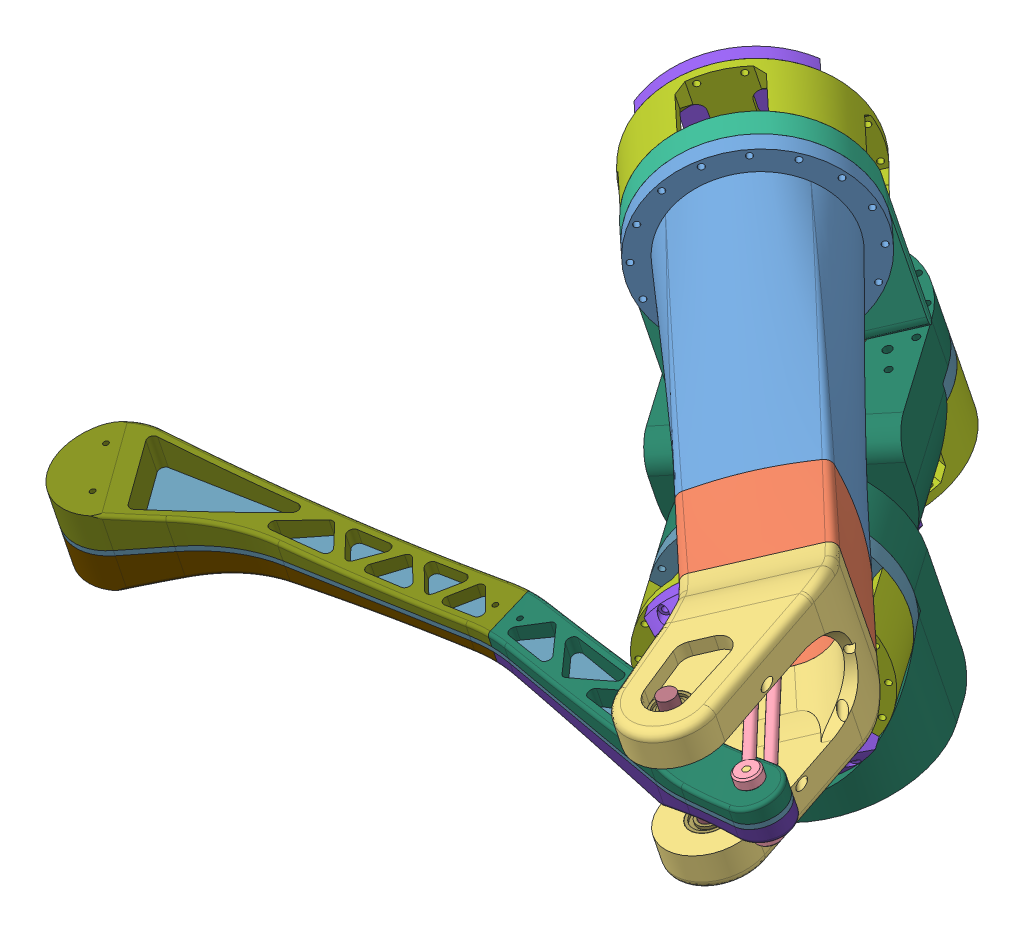
SolidWorks assembly Leg, configuration Default. Lengths in mm.
Overall size (470.99 330.33 460.48).
644 component instances, 120 part files, 60 mates.
Components (placement in the parent):
- ball_screw-1: ball_screw [Default] at (169.6544 226.0363 365.6952) x (0.654638 0.372104 -0.658018) z (0.19821 -0.924497 -0.325604) size (10 178 10)
- ball_screw_slider-1: ball_screw_slider [Default] at (223.929 219.8814 416.2105) x (-0.673603 -0.259208 0.692149) z (-0.118734 0.962272 0.244816) size (45 40.01 30)
- connection_rod_base-1: connection_rod_base [Default] at (223.929 219.8814 416.2105) x (-0.673603 -0.259208 0.692149) z (-0.118734 0.962272 0.244816) size (45 47 45.02)
- Link_Rod-1: Link_Rod [Default] at (251.6245 228.6007 446.4293) x (0.684304 -0.099352 0.722397) z (-0.719465 -0.253302 0.64669) size (214 7 14)
- Link_Rod-2: Link_Rod [Default] at (255.424 197.808 438.5952) x (0.684304 -0.099352 0.722397) z (-0.719465 -0.253302 0.64669) size (214 7 14)
- Shaft Coupler D25L30 8x8.step-1: Shaft Coupler D25L30 8x8.step [Default] at (173.2149 242.8618 353.1431) x (-0.445162 -0.811071 0.379467) z (0.729494 -0.082727 0.678966) size (25 25 30)
  - 8x8_Flexible_Spider_Shaft_Coupling.step-1: 8x8_Flexible_Spider_Shaft_Coupling.step [Default] at origin size (25 25 30)
    - Screw.step-1: Screw.step [Default] at (-0.1468 24 -24) size (5.4 14.9 5.4)
    - Coupler R.step-1: Coupler R.step [Default] at origin size (25 25 20)
    - Plastic.step-1: Plastic.step [Default] at (-0.0052 0 -14) size (21.45 21.45 11)
    - Coupler L.step-1: Coupler L.step [Default] at (-0.0052 0.0052 -24) size (25 25 20)
    - Screw (1).step-1: Screw (1).step [Default] at (30.9948 0.0052 -24) size (14.9 5.4 5.4)
- m8-1: m8 [Default] at (136.0926 229.8406 334.468) x (-0.58022 -0.600489 0.550234) z (0.362193 -0.795342 -0.486053) size (15.01 18.7 13)
- Output_Shaft_holder-1: Output_Shaft_holder [Default] at (131.21 230.396 329.9137) x (-0.100879 -0.994816 -0.012824) z (-0.676507 0.059138 0.734058) size (40 5 40)
- radial ball bearing_68_iso-1: radial ball bearing_68_iso [ISO 15 RBB - 286 - 10,SI,NC,10_68] at (275.7957 213.9995 464.4847) x (0.729494 -0.082727 0.678966) z (-0.296468 0.856323 0.422868) size (5 13 13)
- m10-1: m10 [Default] at (355.5956 148.7793 575.7298) x (-0.945639 -0.184771 0.267632) z (-0.30277 0.19973 -0.9319) size (10 90 10)
- radial ball bearing_68_iso-3: radial ball bearing_68_iso [ISO 15 RBB - 1910 - 10,SI,NC,10_68] at (355.2394 151.6661 576.4643) x (-0.118734 0.962272 0.244816) z (0.248305 0.267502 -0.931014) size (6 22 22)
- radial ball bearing_68_iso-4: radial ball bearing_68_iso [ISO 15 RBB - 1910 - 10,SI,NC,10_68] at (346.928 219.0252 593.6014) x (-0.118734 0.962272 0.244816) z (0.833197 -0.037553 0.5517) size (6 22 22)
- Leg_Lower-1: Leg_Lower [Default] at (8.8341 36.8812 203.9788) x (0.992925 0.115508 0.027547) z (0.00177 -0.246355 0.969178) size (435 46.43 76.27)
  - Leg_Lower_in-1: Leg_Lower_in [Default] at (367.4739 202.5146 333.3401) size (435 3 72.6)
  - Leg_Lower_out_left_1-1: Leg_Lower_out_left_1 [Default] at (367.4739 204.0146 333.3401) size (195.32 15.92 59)
  - Leg_Lower_out_left_2-1: Leg_Lower_out_left_2 [Default] at (367.4739 204.0146 333.3401) size (243.01 21.71 76.27)
  - MirrorLeg_Lower_out_left_1-2: MirrorLeg_Lower_out_left_1 [Default] at (367.4739 201.0146 333.3401) x (1 0 0) z (0 0 -1) size (195.32 15.92 59)
  - MirrorLeg_Lower_out_left_2-2: MirrorLeg_Lower_out_left_2 [Default] at (367.4739 201.0146 333.3401) x (1 0 0) z (0 0 -1) size (243.01 21.71 76.27)
- Leg_upper-1: Leg_upper [Default] at (40.5831 406.0931 409.5805) x (0.673603 0.259208 -0.692149) z (0.118734 -0.962272 -0.244816) size (122.65 362.63 115)
  - leg_upper_infront_1-1: leg_upper_infront_1 [Default] at (70.6458 26.5557 199.3325) size (115 195.7 115)
  - leg_upper_infront_2-1: leg_upper_infront_2 [Default] at (70.6458 26.5557 199.3325) x (0 0 1) z (-1 0 0) size (79.21 54.31 79.21)
  - leg_upper_infront_2_kfe-1: leg_upper_infront_2_kfe [Default] at (70.6458 26.5557 199.3325) x (0 0 -1) z (1 0 0) size (90 112.35 100.44)
  - m5_cacbon-1: m5_cacbon [Default] at (110.6518 26.3844 199.3325) x (0.214067 0.007492 -0.97679) z (0.976192 0.034167 0.214198) size (5 275 5)
  - m5_cacbon-2: m5_cacbon [Default] at (70.6458 26.602 159.3342) x (-0.895778 0.015548 -0.44423) z (0.444502 0.031333 -0.89523) size (5 275 5)
  - m5_cacbon-3: m5_cacbon [Default] at (42.3605 26.5163 227.6178) x (-0.865366 0.009016 -0.50106) z (0.50053 -0.033797 -0.865059) size (5 275 5) (hidden)
  - m5_cacbon-4: m5_cacbon [Default] at (98.9345 26.3769 171.0439) x (0.474029 0.033507 -0.879871) z (0.880162 0.010038 0.474568) size (5 275 5)
  - m5_cacbon-5: m5_cacbon [Default] at (30.6521 26.7357 199.3325) x (-0.639815 0.022394 0.768203) z (-0.767732 0.026871 -0.640207) size (5 275 5) (hidden)
  - m5_cacbon-6: m5_cacbon [Default] at (70.6458 26.7405 239.3261) x (-0.498774 0.030317 0.866202) z (-0.866732 -0.017446 -0.498469) size (5 275 5)
  - m5_cacbon-7: m5_cacbon [Default] at (42.3617 26.5621 171.0484) x (0.047605 -0.025891 0.998531) z (-0.99856 0.02352 0.048216) size (5 275 5) (hidden)
  - m5_cacbon-8: m5_cacbon [Default] at (98.9324 26.4628 227.6191) x (0.999057 0.025593 0.035064) z (-0.035675 0.023843 0.999079) size (5 275 5)
- m4x14-1: m4x14 [Default] at (145.1245 229.0906 321.7269) x (-0.555859 0.506737 0.658968) z (-0.398572 -0.858122 0.323677) size (8 15.2 8)
- kfe_bldc-1: kfe_bldc [Default] at (193.3909 346.3212 344.74) x (-0.673603 -0.259208 0.692149) z (0.118734 -0.962272 -0.244816) size (115 64.6 130.07)
  - cover-1: cover [Default] at (61.6719 45.8369 107.7982) size (115 63.6 130)
  - Motor_Cover_v2-1: Motor_Cover_v2 [Default] at (61.6719 95.4369 107.7982) x (1 0 0) z (0 0 -1) size (115 34.6 115)
  - driver_cover-1: driver_cover [Default] at (61.6719 95.4369 107.7982) x (0.999998 0 0.001745) z (-0.001745 0 0.999998) size (81.32 15 115)
  - Base_Plate_kfe-1: Base_Plate_kfe [Default] at (61.6719 61.3369 107.7982) x (0.999805 0 0.01976) z (0.01976 0 -0.999805) size (40 15.5 40)
  - radial ball bearing_68_iso-2: radial ball bearing_68_iso [ISO 15 RBB - 1840 - 32,SI,NC,32_68] at (61.6719 49.3369 107.7982) x (0 -1 0) z (0 0 1) size (7 52 52)
  - Part1-1: Part1 [Default] at (61.6719 45.8369 107.7982) size (57.8 10 57.8)
- Cycloidal _v3-1: Cycloidal _v3 [Default] at (225.629 71.2826 236.7117) x (-0.201502 -0.265168 0.942912) z (-0.972255 -0.062625 -0.225384) size (173.36 87.57 173.15)
  - motor-X83008S.stp-1: motor-X83008S.stp [Default] at (3.9105 88.7742 94.1058) x (0.928336 0.00037 -0.371741) z (0.000399 -1 0) size (114.7 114.7 37.62) (hidden)
    - base.stp-1: base.stp [Default] at (42.0794 12.0269 46.7342) size (91.6 91.6 15.61)
    - stator.stp-1: stator.stp [Default] at (42.0794 12.0269 33.1342) x (0.08493 -0.996387 0) z (0 0 1) size (83 83 8)
    - coil.stp-1: coil.stp [Default] at (39.5332 41.8984 37.1342) x (0.996387 0.08493 0) z (-0.08493 0.996387 0) size (4.4 10.2 10.5)
    - coil.stp-2: coil.stp [Default] at (34.3848 41.0025 37.1342) x (0.966502 0.256661 0) z (-0.256661 0.966502 0) size (4.4 10.2 10.5)
    - coil.stp-3: coil.stp [Default] at (29.4701 39.2261 37.1342) x (0.90725 0.420593 0) z (-0.420593 0.90725 0) size (4.4 10.2 10.5)
    - coil.stp-4: coil.stp [Default] at (24.9386 36.6233 37.1342) x (0.820431 0.571745 0) z (-0.571745 0.820431 0) size (4.4 10.2 10.5)
    - coil.stp-5: coil.stp [Default] at (20.9279 33.2732 37.1342) x (0.708685 0.705525 0) z (-0.705525 0.708685 0) size (4.4 10.2 10.5)
    - coil.stp-6: coil.stp [Default] at (17.5599 29.2775 37.1342) x (0.575405 0.817869 0) z (-0.817869 0.575405 0) size (4.4 10.2 10.5)
    - coil.stp-7: coil.stp [Default] at (14.9368 24.7576 37.1342) x (0.424642 0.905361 0) z (-0.905361 0.424642 0) size (4.4 10.2 10.5)
    - coil.stp-8: coil.stp [Default] at (13.1385 19.8509 37.1342) x (0.260976 0.965345 0) z (-0.965345 0.260976 0) size (4.4 10.2 10.5)
    - coil.stp-9: coil.stp [Default] at (12.2196 14.7066 37.1342) x (0.089381 0.995998 0) z (-0.995998 0.089381 0) size (4.4 10.2 10.5)
    - coil.stp-10: coil.stp [Default] at (12.2079 9.4807 37.1342) x (-0.08493 0.996387 0) z (-0.996387 -0.08493 0) size (4.4 10.2 10.5)
    - coil.stp-11: coil.stp [Default] at (13.1039 4.3323 37.1342) x (-0.256661 0.966502 0) z (-0.966502 -0.256661 0) size (4.4 10.2 10.5)
    - coil.stp-12: coil.stp [Default] at (14.8802 -0.5824 37.1342) x (-0.420593 0.90725 0) z (-0.90725 -0.420593 0) size (4.4 10.2 10.5)
    - coil.stp-13: coil.stp [Default] at (17.483 -5.1139 37.1342) x (-0.571745 0.820431 0) z (-0.820431 -0.571745 0) size (4.4 10.2 10.5)
    - coil.stp-14: coil.stp [Default] at (20.8332 -9.1246 37.1342) x (-0.705525 0.708685 0) z (-0.708685 -0.705525 0) size (4.4 10.2 10.5)
    - coil.stp-15: coil.stp [Default] at (24.8289 -12.4926 37.1342) x (-0.817869 0.575405 0) z (-0.575405 -0.817869 0) size (4.4 10.2 10.5)
    - coil.stp-16: coil.stp [Default] at (29.3487 -15.1157 37.1342) x (-0.905361 0.424642 0) z (-0.424642 -0.905361 0) size (4.4 10.2 10.5)
    - coil.stp-17: coil.stp [Default] at (34.2554 -16.914 37.1342) x (-0.965345 0.260976 0) z (-0.260976 -0.965345 0) size (4.4 10.2 10.5)
    - coil.stp-18: coil.stp [Default] at (39.3998 -17.8329 37.1342) x (-0.995998 0.089381 0) z (-0.089381 -0.995998 0) size (4.4 10.2 10.5)
    - coil.stp-19: coil.stp [Default] at (44.6256 -17.8446 37.1342) x (-0.996387 -0.08493 0) z (0.08493 -0.996387 0) size (4.4 10.2 10.5)
    - coil.stp-20: coil.stp [Default] at (49.7741 -16.9486 37.1342) x (-0.966502 -0.256661 0) z (0.256661 -0.966502 0) size (4.4 10.2 10.5)
    - coil.stp-21: coil.stp [Default] at (54.6887 -15.1723 37.1342) x (-0.90725 -0.420593 0) z (0.420593 -0.90725 0) size (4.4 10.2 10.5)
    - coil.stp-22: coil.stp [Default] at (59.2202 -12.5695 37.1342) x (-0.820431 -0.571745 0) z (0.571745 -0.820431 0) size (4.4 10.2 10.5)
    - coil.stp-23: coil.stp [Default] at (63.2309 -9.2193 37.1342) x (-0.708685 -0.705525 0) z (0.705525 -0.708685 0) size (4.4 10.2 10.5)
    - coil.stp-24: coil.stp [Default] at (66.599 -5.2236 37.1342) x (-0.575405 -0.817869 0) z (0.817869 -0.575405 0) size (4.4 10.2 10.5)
    - coil.stp-25: coil.stp [Default] at (69.222 -0.7038 37.1342) x (-0.424642 -0.905361 0) z (0.905361 -0.424642 0) size (4.4 10.2 10.5)
    - coil.stp-26: coil.stp [Default] at (71.0203 4.2029 37.1342) x (-0.260976 -0.965345 0) z (0.965345 -0.260976 0) size (4.4 10.2 10.5)
    - coil.stp-27: coil.stp [Default] at (71.9392 9.3473 37.1342) x (-0.089381 -0.995998 0) z (0.995998 -0.089381 0) size (4.4 10.2 10.5)
    - coil.stp-28: coil.stp [Default] at (71.9509 14.5731 37.1342) x (0.08493 -0.996387 0) z (0.996387 0.08493 0) size (4.4 10.2 10.5)
    - coil.stp-29: coil.stp [Default] at (71.055 19.7216 37.1342) x (0.256661 -0.966502 0) z (0.966502 0.256661 0) size (4.4 10.2 10.5)
    - coil.stp-30: coil.stp [Default] at (69.2786 24.6362 37.1342) x (0.420593 -0.90725 0) z (0.90725 0.420593 0) size (4.4 10.2 10.5)
    - coil.stp-31: coil.stp [Default] at (66.6758 29.1677 37.1342) x (0.571745 -0.820431 0) z (0.820431 0.571745 0) size (4.4 10.2 10.5)
    - coil.stp-32: coil.stp [Default] at (63.3257 33.1785 37.1342) x (0.705525 -0.708685 0) z (0.708685 0.705525 0) size (4.4 10.2 10.5)
    - coil.stp-33: coil.stp [Default] at (59.33 36.5465 37.1342) x (0.817869 -0.575405 0) z (0.575405 0.817869 0) size (4.4 10.2 10.5)
    - coil.stp-34: coil.stp [Default] at (54.8101 39.1695 37.1342) x (0.905361 -0.424642 0) z (0.424642 0.905361 0) size (4.4 10.2 10.5)
    - coil.stp-35: coil.stp [Default] at (49.9034 40.9678 37.1342) x (0.965345 -0.260976 0) z (0.260976 0.965345 0) size (4.4 10.2 10.5)
    - coil.stp-36: coil.stp [Default] at (44.759 41.8868 37.1342) x (0.995998 -0.089381 0) z (0.089381 0.995998 0) size (4.4 10.2 10.5)
    - rotor.stp-1: rotor.stp [Default] at (42.0794 12.0269 42.1342) x (-0.293442 0.955977 0) z (0 0 -1) size (91.8 91.8 12)
    - outrunner.stp-1: outrunner.stp [Default] at (42.0794 12.0269 30.1342) x (-0.254711 0.967017 0) z (-0.967017 -0.254711 0) size (91.8 17.01 91.8)
    - screw-mount.stp-1: screw-mount.stp [Default] at (38.1314 27.0157 27.1342) x (1 0 0) z (0 0 -1) size (7 7 6.5)
    - screw-mount.stp-2: screw-mount.stp [Default] at (27.0906 8.0789 27.1342) x (1 0 0) z (0 0 -1) size (7 7 6.5)
    - screw-mount.stp-3: screw-mount.stp [Default] at (57.0682 15.9749 27.1342) x (1 0 0) z (0 0 -1) size (7 7 6.5)
    - screw-mount.stp-4: screw-mount.stp [Default] at (46.0274 -2.9618 27.1342) x (1 0 0) z (0 0 -1) size (7 7 6.5)
    - 6702ZZ-bearing-15x21x4.stp-1: 6702ZZ-bearing-15x21x4.stp [Default] at (42.0794 12.0269 43.7342) x (1 0 0) z (0 -1 0) size (21 4 21)
    - 6702ZZ-bearing-15x21x4.stp-2: 6702ZZ-bearing-15x21x4.stp [Default] at (42.0794 12.0269 35.1342) x (1 0 0) z (0 1 0) size (21 4 21)
    - shaft.stp-1: shaft.stp [Default] at (42.0794 12.0269 20.1342) size (16 16 31.6)
    - fix-screw.stp-1: fix-screw.stp [Default] at (42.0794 12.0269 51.7342) x (1 0 0) z (0 0 -1) size (19.67 18.96 12.02)
  - Base_Plate-1: Base_Plate [Default] at (47.4533 68.6574 89.6282) x (-0.992404 -0.000396 0.123023) z (-0.123023 -0.000049 -0.992404) size (39.8 11 39.8)
  - Eccentric_Shaft-1: Eccentric_Shaft [Default] at (60.4961 73.3217 80.3225) x (0.123023 0.000049 0.992404) z (-0.992404 -0.000396 0.123023) size (20 17 17)
    - Eccentric_Shaft_bot-1: Eccentric_Shaft_bot [Default] at (7.6302 12.3409 14.0904) x (1 0 0) z (0 0 -1) size (17 6 17)
    - Eccentric_Shaft_bot-2: Eccentric_Shaft_bot [Default] at (7.6302 12.3409 14.0904) x (-1 0 0) z (0 0 -1) size (17 6 17)
    - Eccentric_Shaft_top-1: Eccentric_Shaft_top [Default] at (7.6302 18.3409 14.0904) x (-1 0 0) z (0 0 -1) size (17 5 17)
  - radial ball bearing_68_iso-39: radial ball bearing_68_iso [ISO 15 RBB - 1860 - 32,SI,NC,32_68] at (47.4409 99.6574 89.6282) x (0.000399 -1 0) z (-0.546908 -0.000218 0.837193) size (10 78 78)
  - radial ball bearing_68_iso-40: radial ball bearing_68_iso [ISO 15 RBB - 1840 - 32,SI,NC,32_68] at (47.4516 72.9574 89.6282) x (-0.000399 1 0) z (0.001003 0 0.999999) size (7 52 52)
  - Base_plate_2-1: Base_plate_2 [Default] at (47.4529 69.6574 89.6282) x (0.712755 0.000284 -0.701413) z (0.701413 0.00028 0.712755) size (115 10 115)
  - m13_bearing-31: m13_bearing [Default] at (-10.4263 95.4017 67.196) x (0.227678 0.000091 0.973736) z (0.973736 0.000388 -0.227678) size (13 16 13)
    - m6-1: m6 [Default] at (8.4921 2.5508 14.8914) size (6 16 6)
    - radial ball bearing_68_iso-1: radial ball bearing_68_iso [ISO 15 RBB - 286 - 10,SI,NC,10_68] at (8.4921 16.0508 14.8914) x (0 1 0) z (0 0 1) size (5 13 13)
    - radial ball bearing_68_iso-2: radial ball bearing_68_iso [ISO 15 RBB - 286 - 10,SI,NC,10_68] at (8.4921 11.0508 14.8914) x (0 1 0) z (0 0 1) size (5 13 13)
  - m13_bearing-32: m13_bearing [Default] at (-13.9908 98.1837 84.3887) x (0.227678 0.000091 0.973736) z (0.973736 0.000388 -0.227678) size (13 16 13)
    - m6-1: m6 [Default] at (8.4921 2.5508 14.8914) size (6 16 6)
    - radial ball bearing_68_iso-1: radial ball bearing_68_iso [ISO 15 RBB - 286 - 10,SI,NC,10_68] at (8.4921 16.0508 14.8914) x (0 1 0) z (0 0 1) size (5 13 13)
    - radial ball bearing_68_iso-2: radial ball bearing_68_iso [ISO 15 RBB - 286 - 10,SI,NC,10_68] at (8.4921 11.0508 14.8914) x (0 1 0) z (0 0 1) size (5 13 13)
  - m13_bearing-34: m13_bearing [Default] at (13.4541 98.1947 126.1847) x (0.227678 0.000091 0.973736) z (0.973736 0.000388 -0.227678) size (13 16 13)
    - m6-1: m6 [Default] at (8.4921 2.5508 14.8914) size (6 16 6)
    - radial ball bearing_68_iso-1: radial ball bearing_68_iso [ISO 15 RBB - 286 - 10,SI,NC,10_68] at (8.4921 16.0508 14.8914) x (0 1 0) z (0 0 1) size (5 13 13)
    - radial ball bearing_68_iso-2: radial ball bearing_68_iso [ISO 15 RBB - 286 - 10,SI,NC,10_68] at (8.4921 11.0508 14.8914) x (0 1 0) z (0 0 1) size (5 13 13)
  - m13_bearing-35: m13_bearing [Default] at (-1.0662 98.1889 116.3132) x (0.227678 0.000091 0.973736) z (0.973736 0.000388 -0.227678) size (13 16 13)
    - m6-1: m6 [Default] at (8.4921 2.5508 14.8914) size (6 16 6)
    - radial ball bearing_68_iso-1: radial ball bearing_68_iso [ISO 15 RBB - 286 - 10,SI,NC,10_68] at (8.4921 16.0508 14.8914) x (0 1 0) z (0 0 1) size (5 13 13)
    - radial ball bearing_68_iso-2: radial ball bearing_68_iso [ISO 15 RBB - 286 - 10,SI,NC,10_68] at (8.4921 11.0508 14.8914) x (0 1 0) z (0 0 1) size (5 13 13)
  - m13_bearing-36: m13_bearing [Default] at (-10.7036 98.185 101.6364) x (0.227678 0.000091 0.973736) z (0.973736 0.000388 -0.227678) size (13 16 13)
    - m6-1: m6 [Default] at (8.4921 2.5508 14.8914) size (6 16 6)
    - radial ball bearing_68_iso-1: radial ball bearing_68_iso [ISO 15 RBB - 286 - 10,SI,NC,10_68] at (8.4921 16.0508 14.8914) x (0 1 0) z (0 0 1) size (5 13 13)
    - radial ball bearing_68_iso-2: radial ball bearing_68_iso [ISO 15 RBB - 286 - 10,SI,NC,10_68] at (8.4921 11.0508 14.8914) x (0 1 0) z (0 0 1) size (5 13 13)
  - m13_bearing-1: m13_bearing [Default] at (-0.4494 98.1891 62.778) x (0.736525 0.000294 0.676411) z (0.676411 0.00027 -0.736525) size (13 16 13)
    - m6-1: m6 [Default] at (8.4921 2.5508 14.8914) size (6 16 6)
    - radial ball bearing_68_iso-1: radial ball bearing_68_iso [ISO 15 RBB - 286 - 10,SI,NC,10_68] at (8.4921 16.0508 14.8914) x (0 1 0) z (0 0 1) size (5 13 13)
    - radial ball bearing_68_iso-2: radial ball bearing_68_iso [ISO 15 RBB - 286 - 10,SI,NC,10_68] at (8.4921 11.0508 14.8914) x (0 1 0) z (0 0 1) size (5 13 13)
  - m13_bearing-2: m13_bearing [Default] at (48.5236 98.2087 124.7001) x (0.120271 0.000048 0.992741) z (0.992741 0.000396 -0.120271) size (13 16 13)
    - m6-1: m6 [Default] at (8.4921 2.5508 14.8914) size (6 16 6)
    - radial ball bearing_68_iso-1: radial ball bearing_68_iso [ISO 15 RBB - 286 - 10,SI,NC,10_68] at (8.4921 16.0508 14.8914) x (0 1 0) z (0 0 1) size (5 13 13)
    - radial ball bearing_68_iso-2: radial ball bearing_68_iso [ISO 15 RBB - 286 - 10,SI,NC,10_68] at (8.4921 11.0508 14.8914) x (0 1 0) z (0 0 1) size (5 13 13)
  - m13_bearing-3: m13_bearing [Default] at (32.5019 98.2023 52.3604) x (0.833889 0.000333 0.551933) z (0.551932 0.00022 -0.833889) size (13 16 13)
    - m6-1: m6 [Default] at (8.4921 2.5508 14.8914) size (6 16 6)
    - radial ball bearing_68_iso-1: radial ball bearing_68_iso [ISO 15 RBB - 286 - 10,SI,NC,10_68] at (8.4921 16.0508 14.8914) x (0 1 0) z (0 0 1) size (5 13 13)
    - radial ball bearing_68_iso-2: radial ball bearing_68_iso [ISO 15 RBB - 286 - 10,SI,NC,10_68] at (8.4921 11.0508 14.8914) x (0 1 0) z (0 0 1) size (5 13 13)
  - m13_bearing-4: m13_bearing [Default] at (77.3632 98.2202 81.8307) x (0.022268 0.000009 0.999752) z (0.999752 0.000399 -0.022268) size (13 16 13)
    - m6-1: m6 [Default] at (8.4921 2.5508 14.8914) size (6 16 6)
    - radial ball bearing_68_iso-1: radial ball bearing_68_iso [ISO 15 RBB - 286 - 10,SI,NC,10_68] at (8.4921 16.0508 14.8914) x (0 1 0) z (0 0 1) size (5 13 13)
    - radial ball bearing_68_iso-2: radial ball bearing_68_iso [ISO 15 RBB - 286 - 10,SI,NC,10_68] at (8.4921 11.0508 14.8914) x (0 1 0) z (0 0 1) size (5 13 13)
  - m13_bearing-5: m13_bearing [Default] at (73.5091 98.2186 99.5852) x (0.059133 0.000024 0.99825) z (0.99825 0.000398 -0.059133) size (13 16 13)
    - m6-1: m6 [Default] at (8.4921 2.5508 14.8914) size (6 16 6)
    - radial ball bearing_68_iso-1: radial ball bearing_68_iso [ISO 15 RBB - 286 - 10,SI,NC,10_68] at (8.4921 16.0508 14.8914) x (0 1 0) z (0 0 1) size (5 13 13)
    - radial ball bearing_68_iso-2: radial ball bearing_68_iso [ISO 15 RBB - 286 - 10,SI,NC,10_68] at (8.4921 11.0508 14.8914) x (0 1 0) z (0 0 1) size (5 13 13)
  - m13_bearing-6: m13_bearing [Default] at (13.4333 98.1947 47.0643) x (0.451561 0.00018 0.89224) z (0.89224 0.000356 -0.451561) size (13 16 13)
    - m6-1: m6 [Default] at (8.4921 2.5508 14.8914) size (6 16 6)
    - radial ball bearing_68_iso-1: radial ball bearing_68_iso [ISO 15 RBB - 286 - 10,SI,NC,10_68] at (8.4921 16.0508 14.8914) x (0 1 0) z (0 0 1) size (5 13 13)
    - radial ball bearing_68_iso-2: radial ball bearing_68_iso [ISO 15 RBB - 286 - 10,SI,NC,10_68] at (8.4921 11.0508 14.8914) x (0 1 0) z (0 0 1) size (5 13 13)
  - m13_bearing-7: m13_bearing [Default] at (57.1526 98.2121 32.9496) x (-0.545813 -0.000218 0.837907) z (0.837907 0.000334 0.545813) size (13 16 13)
    - m6-1: m6 [Default] at (8.4921 2.5508 14.8914) size (6 16 6)
    - radial ball bearing_68_iso-1: radial ball bearing_68_iso [ISO 15 RBB - 286 - 10,SI,NC,10_68] at (8.4921 16.0508 14.8914) x (0 1 0) z (0 0 1) size (5 13 13)
    - radial ball bearing_68_iso-2: radial ball bearing_68_iso [ISO 15 RBB - 286 - 10,SI,NC,10_68] at (8.4921 11.0508 14.8914) x (0 1 0) z (0 0 1) size (5 13 13)
  - m13_bearing-8: m13_bearing [Default] at (73.1034 98.2185 66.7178) x (0.158553 0.000063 0.98735) z (0.98735 0.000394 -0.158553) size (13 16 13)
    - m6-1: m6 [Default] at (8.4921 2.5508 14.8914) size (6 16 6)
    - radial ball bearing_68_iso-1: radial ball bearing_68_iso [ISO 15 RBB - 286 - 10,SI,NC,10_68] at (8.4921 16.0508 14.8914) x (0 1 0) z (0 0 1) size (5 13 13)
    - radial ball bearing_68_iso-2: radial ball bearing_68_iso [ISO 15 RBB - 286 - 10,SI,NC,10_68] at (8.4921 11.0508 14.8914) x (0 1 0) z (0 0 1) size (5 13 13)
  - m13_bearing-9: m13_bearing [Default] at (74.5316 98.219 41.6624) x (-0.687134 -0.000274 0.72653) z (0.72653 0.00029 0.687134) size (13 16 13)
    - m6-1: m6 [Default] at (8.4921 2.5508 14.8914) size (6 16 6)
    - radial ball bearing_68_iso-1: radial ball bearing_68_iso [ISO 15 RBB - 286 - 10,SI,NC,10_68] at (8.4921 16.0508 14.8914) x (0 1 0) z (0 0 1) size (5 13 13)
    - radial ball bearing_68_iso-2: radial ball bearing_68_iso [ISO 15 RBB - 286 - 10,SI,NC,10_68] at (8.4921 11.0508 14.8914) x (0 1 0) z (0 0 1) size (5 13 13)
  - m13_bearing-11: m13_bearing [Default] at (30.0113 98.2013 136.2104) x (0.57351 0.000229 0.819198) z (0.819198 0.000327 -0.57351) size (13 16 13)
    - m6-1: m6 [Default] at (8.4921 2.5508 14.8914) size (6 16 6)
    - radial ball bearing_68_iso-1: radial ball bearing_68_iso [ISO 15 RBB - 286 - 10,SI,NC,10_68] at (8.4921 16.0508 14.8914) x (0 1 0) z (0 0 1) size (5 13 13)
    - radial ball bearing_68_iso-2: radial ball bearing_68_iso [ISO 15 RBB - 286 - 10,SI,NC,10_68] at (8.4921 11.0508 14.8914) x (0 1 0) z (0 0 1) size (5 13 13)
  - m13_bearing-12: m13_bearing [Default] at (62.5932 98.2143 116.7506) x (0.22335 0.000089 0.974738) z (0.974738 0.000389 -0.22335) size (13 16 13)
    - m6-1: m6 [Default] at (8.4921 2.5508 14.8914) size (6 16 6)
    - radial ball bearing_68_iso-1: radial ball bearing_68_iso [ISO 15 RBB - 286 - 10,SI,NC,10_68] at (8.4921 16.0508 14.8914) x (0 1 0) z (0 0 1) size (5 13 13)
    - radial ball bearing_68_iso-2: radial ball bearing_68_iso [ISO 15 RBB - 286 - 10,SI,NC,10_68] at (8.4921 11.0508 14.8914) x (0 1 0) z (0 0 1) size (5 13 13)
  - M3x4x4.2_brass_insert-22: M3x4x4.2_brass_insert [Default] at (43.4837 68.6558 90.1203) x (0.984609 0.000393 -0.174769) z (0.174769 0.00007 0.984609) size (4 4 4)
  - M3x4x4.2_brass_insert-23: M3x4x4.2_brass_insert [Default] at (51.4229 68.659 89.1361) x (0.984609 0.000393 -0.174769) z (0.174769 0.00007 0.984609) size (4 4 4)
  - radial ball bearing_68_iso-44: radial ball bearing_68_iso [ISO 15 RBB - 1715 - 26,SI,NC,26_68] at (47.2636 81.6573 88.1396) x (0.000399 -1 0) z (0.171535 0.000068 0.985178) size (4 21 21)
  - radial ball bearing_68_iso-45: radial ball bearing_68_iso [ISO 15 RBB - 1715 - 26,SI,NC,26_68] at (47.4429 94.6574 89.6282) x (0.000399 -1 0) z (0.819169 0.000327 0.573552) size (4 21 21)
  - radial ball bearing_68_iso-46: radial ball bearing_68_iso [ISO 15 RBB - 1715 - 26,SI,NC,26_68] at (47.6295 89.6575 91.1168) x (-0.000399 1 0) z (0 0 1) size (4 21 21)
  - foc-motor-controller.step-1: foc-motor-controller.step [Default] at (47.4677 32.6574 89.6282) x (0.701413 0.00028 0.712755) z (0.000399 -1 0) size (57.23 50 8.13)
    - RTA0040B.step-1: RTA0040B.step [Default] at (12.5014 -1.6986 1.595) x (-0.707107 -0.707107 0) z (0 0 1) size (6 6 1)
      - FRAME.step-1: FRAME.step [Default] x (1 0 0) z (0 -1 0) size (6 0.2 6)
        - SOLID.step-1: SOLID.step [Default] at origin size (0.4 0.2 0.22)
        - SOLID-0.step-1: SOLID-0.step [Default] at origin size (0.4 0.2 0.22)
        - SOLID-1.step-1: SOLID-1.step [Default] at origin size (0.4 0.2 0.22)
        - SOLID-2.step-1: SOLID-2.step [Default] at origin size (0.4 0.2 0.22)
        - SOLID-3.step-1: SOLID-3.step [Default] at origin size (0.4 0.2 0.22)
        - SOLID-4.step-1: SOLID-4.step [Default] at origin size (0.4 0.2 0.22)
        - SOLID-5.step-1: SOLID-5.step [Default] at origin size (0.4 0.2 0.22)
        - SOLID-6.step-1: SOLID-6.step [Default] at origin size (0.4 0.2 0.22)
        - SOLID-7.step-1: SOLID-7.step [Default] at origin size (0.4 0.2 0.22)
        - SOLID-8.step-1: SOLID-8.step [Default] at origin size (0.4 0.2 0.22)
        - SOLID-9.step-1: SOLID-9.step [Default] at origin size (0.22 0.2 0.4)
        - SOLID-10.step-1: SOLID-10.step [Default] at origin size (0.22 0.2 0.4)
        - SOLID-11.step-1: SOLID-11.step [Default] at origin size (0.22 0.2 0.4)
        - SOLID-12.step-1: SOLID-12.step [Default] at origin size (0.22 0.2 0.4)
        - SOLID-13.step-1: SOLID-13.step [Default] at origin size (0.22 0.2 0.4)
        - SOLID-14.step-1: SOLID-14.step [Default] at origin size (0.22 0.2 0.4)
        - SOLID-15.step-1: SOLID-15.step [Default] at origin size (0.22 0.2 0.4)
        - SOLID-16.step-1: SOLID-16.step [Default] at origin size (0.22 0.2 0.4)
        - SOLID-17.step-1: SOLID-17.step [Default] at origin size (4.15 0.2 4.15)
        - SOLID-18.step-1: SOLID-18.step [Default] at origin size (0.28 0.1 0.28)
        - SOLID-19.step-1: SOLID-19.step [Default] at origin size (0.28 0.1 0.28)
        - SOLID-20.step-1: SOLID-20.step [Default] at origin size (0.28 0.1 0.28)
        - SOLID-21.step-1: SOLID-21.step [Default] at origin size (0.28 0.1 0.28)
        - SOLID-22.step-1: SOLID-22.step [Default] at origin size (0.4 0.2 0.22)
        - SOLID-23.step-1: SOLID-23.step [Default] at origin size (0.4 0.2 0.22)
        - SOLID-24.step-1: SOLID-24.step [Default] at origin size (0.4 0.2 0.22)
        - SOLID-25.step-1: SOLID-25.step [Default] at origin size (0.4 0.2 0.22)
        - SOLID-26.step-1: SOLID-26.step [Default] at origin size (0.4 0.2 0.22)
        - SOLID-27.step-1: SOLID-27.step [Default] at origin size (0.4 0.2 0.22)
        - SOLID-28.step-1: SOLID-28.step [Default] at origin size (0.4 0.2 0.22)
        - SOLID-29.step-1: SOLID-29.step [Default] at origin size (0.4 0.2 0.22)
        - SOLID-30.step-1: SOLID-30.step [Default] at origin size (0.4 0.2 0.22)
        - SOLID-31.step-1: SOLID-31.step [Default] at origin size (0.4 0.2 0.22)
        - SOLID-32.step-1: SOLID-32.step [Default] at origin size (0.22 0.2 0.4)
        - SOLID-33.step-1: SOLID-33.step [Default] at origin size (0.22 0.2 0.4)
        - SOLID-34.step-1: SOLID-34.step [Default] at origin size (0.22 0.2 0.4)
        - SOLID-35.step-1: SOLID-35.step [Default] at origin size (0.22 0.2 0.4)
        - SOLID-36.step-1: SOLID-36.step [Default] at origin size (0.22 0.2 0.4)
        - SOLID-37.step-1: SOLID-37.step [Default] at origin size (0.22 0.2 0.4)
        - SOLID-38.step-1: SOLID-38.step [Default] at origin size (0.22 0.2 0.4)
        - SOLID-39.step-1: SOLID-39.step [Default] at origin size (0.22 0.2 0.4)
        - SOLID-40.step-1: SOLID-40.step [Default] at origin size (0.22 0.2 0.4)
        - SOLID-41.step-1: SOLID-41.step [Default] at origin size (0.22 0.2 0.4)
        - SOLID-42.step-1: SOLID-42.step [Default] at origin size (0.22 0.2 0.4)
        - SOLID-43.step-1: SOLID-43.step [Default] at origin size (0.22 0.2 0.4)
      - BODY.step-1: BODY.step [Default] at (0 0 0.025) x (1 0 0) z (0 -1 0) size (6 0.97 6)
    - Resonator_SMD_Murata_CSTxExxV-3Pin_3.0x1.1mm.step-1: Resonator_SMD_Murata_CSTxExxV-3Pin_3.0x1.1mm.step [Default] at (1.8 -7 1.595) x (0 1 0) z (0 0 1) size (3.2 1.35 0.9)
    - C_0603_1608Metric.step-1: C_0603_1608Metric.step [Default] at (6.2 -16.8 1.595) x (0 -1 0) z (0 0 1) size (1.6 0.8 0.8)
    - R_0603_1608Metric.step-1: R_0603_1608Metric.step [Default] at (11.8 -7.375 1.595) x (0 1 0) z (0 0 1) size (1.6 0.8 0.45)
    - R_0603_1608Metric.step-2: R_0603_1608Metric.step [Default] at (13.8 -16.8 1.595) x (0 1 0) z (0 0 1) size (1.6 0.8 0.45)
    - R_0603_1608Metric.step-3: R_0603_1608Metric.step [Default] at (18.1 -5.36 1.595) size (1.6 0.8 0.45)
    - C_0603_1608Metric.step-2: C_0603_1608Metric.step [Default] at (2.6 -0.5 1.595) x (0 -1 0) z (0 0 1) size (1.6 0.8 0.8)
    - R_0603_1608Metric.step-4: R_0603_1608Metric.step [Default] at (14.6 -11.3 1.595) x (0 1 0) z (0 0 1) size (1.6 0.8 0.45)
    - L_APV_ANR4020.step-1: L_APV_ANR4020.step [Default] at (22.3 -13.7 1.595) x (0 -1 0) z (0 0 1) size (4.02 4 2)
    - C_0603_1608Metric.step-3: C_0603_1608Metric.step [Default] at (0.3 -12.6 1.595) x (-1 0 0) z (0 0 1) size (1.6 0.8 0.8)
    - C_1206_3216Metric.step-1: C_1206_3216Metric.step [Default] at (15.7 11 1.595) x (0 1 0) z (0 0 1) size (3.2 1.6 1.6)
    - C_0603_1608Metric.step-4: C_0603_1608Metric.step [Default] at (0.3 -9.6 1.595) size (1.6 0.8 0.8)
    - R_0603_1608Metric.step-5: R_0603_1608Metric.step [Default] at (12.3 -16.8 1.595) x (0 1 0) z (0 0 1) size (1.6 0.8 0.45)
    - C_0603_1608Metric.step-5: C_0603_1608Metric.step [Default] at (-0.3 -16.6 1.595) x (0 1 0) z (0 0 1) size (1.6 0.8 0.8)
    - R_0603_1608Metric.step-6: R_0603_1608Metric.step [Default] at (10.9 4.1 1.595) size (1.6 0.8 0.45)
    - C_1206_3216Metric.step-2: C_1206_3216Metric.step [Default] at (6.3 11 1.595) x (0 1 0) z (0 0 1) size (3.2 1.6 1.6)
    - XT30PW_2_2_-M.G.B.step-1: XT30PW_2_2_-M.G.B.step [Default] at (-20.5 9.5 1.595) x (0 -1 0) z (-1 0 0) size (15.5 7.1 12.53)
    - R_0603_1608Metric.step-7: R_0603_1608Metric.step [Default] at (0.3 -11.1 1.595) size (1.6 0.8 0.45)
    - C_0603_1608Metric.step-6: C_0603_1608Metric.step [Default] at (19 -0.4 1.595) x (-0.707107 -0.707107 0) z (0 0 1) size (1.6 0.8 0.8)
    - C_1206_3216Metric.step-3: C_1206_3216Metric.step [Default] at (13.3 11 1.595) x (0 1 0) z (0 0 1) size (3.2 1.6 1.6)
    - R_0603_1608Metric.step-8: R_0603_1608Metric.step [Default] at (10.2 -7.375 1.595) x (0 -1 0) z (0 0 1) size (1.6 0.8 0.45)
    - JST_GH_SM08B-GHS-TB_1x08-1MP_P1.25mm_Horizontal.step-1: JST_GH_SM08B-GHS-TB_1x08-1MP_P1.25mm_Horizontal.step [Default] at (10 -22 1.595) size (13.25 4.95 4.25)
    - C_1206_3216Metric.step-4: C_1206_3216Metric.step [Default] at (-12.3 11 1.595) x (0 1 0) z (0 0 1) size (3.2 1.6 1.6)
    - JST_GH_SM06B-GHS-TB_1x06-1MP_P1.25mm_Horizontal.step-1: JST_GH_SM06B-GHS-TB_1x06-1MP_P1.25mm_Horizontal.step [Default] at (-4.3 -22 1.595) size (10.75 4.95 4.25)
    - C_0603_1608Metric.step-7: C_0603_1608Metric.step [Default] at (7.3 -4.5 1.595) x (-1 0 0) z (0 0 1) size (1.6 0.8 0.8)
    - R_0603_1608Metric.step-9: R_0603_1608Metric.step [Default] at (18.1 -3.86 1.595) x (-1 0 0) z (0 0 1) size (1.6 0.8 0.45)
    - C_1206_3216Metric.step-5: C_1206_3216Metric.step [Default] at (22.6794 -1.2206 1.595) x (0.707107 -0.707107 0) z (0 0 1) size (3.2 1.6 1.6)
    - R_Array_Convex_4x0402.step-1: R_Array_Convex_4x0402.step [Default] at (6.8 -2.5 1.595) size (1 2 0.35)
    - R_0603_1608Metric.step-10: R_0603_1608Metric.step [Default] at (7.7 -16.8 1.595) x (0 -1 0) z (0 0 1) size (1.6 0.8 0.45)
    - C_1206_3216Metric.step-6: C_1206_3216Metric.step [Default] at (8.7 11 1.595) x (0 1 0) z (0 0 1) size (3.2 1.6 1.6)
    - C_0603_1608Metric.step-8: C_0603_1608Metric.step [Default] at (16.1 -11.3 1.595) x (0 1 0) z (0 0 1) size (1.6 0.8 0.8)
    - SOT-23-5.step-1: SOT-23-5.step [Default] at (-3.1 -16.6 1.595) x (-1 0 0) z (0 0 1) size (2.8 2.9 1.55)
    - C_0603_1608Metric.step-9: C_0603_1608Metric.step [Default] at (17.8 -13.6 1.595) size (1.6 0.8 0.8)
    - R_0603_1608Metric.step-11: R_0603_1608Metric.step [Default] at (-11.5 -20.3875 1.595) x (0 -1 0) z (0 0 1) size (1.6 0.8 0.45)
    - C_0603_1608Metric.step-10: C_0603_1608Metric.step [Default] at (-12.4 2.3 1.595) x (0 1 0) z (0 0 1) size (1.6 0.8 0.8)
    - C_1206_3216Metric.step-7: C_1206_3216Metric.step [Default] at (18 11 1.595) x (0 1 0) z (0 0 1) size (3.2 1.6 1.6)
    - R_0603_1608Metric.step-12: R_0603_1608Metric.step [Default] at (-10.8105 -14.9971 1.595) x (-1 0 0) z (0 0 1) size (1.6 0.8 0.45)
    - C_0603_1608Metric.step-11: C_0603_1608Metric.step [Default] at (-13.8 -9.4 1.595) x (-1 0 0) z (0 0 1) size (1.6 0.8 0.8)
    - R_0603_1608Metric.step-13: R_0603_1608Metric.step [Default] at (-23.15 -14.5 1.595) x (-1 0 0) z (0 0 1) size (1.6 0.8 0.45)
    - C_0603_1608Metric.step-12: C_0603_1608Metric.step [Default] at (1.1 -0.2 1.595) x (0 1 0) z (0 0 1) size (1.6 0.8 0.8)
    - D_0805_2012Metric.step-1: D_0805_2012Metric.step [Default] at (22.9 -9.6 1.595) x (0 1 0) z (0 0 1) size (2 1.27 0.8)
    - C_0603_1608Metric.step-13: C_0603_1608Metric.step [Default] at (-7.8 3.775 1.595) x (0 -1 0) z (0 0 1) size (1.6 0.8 0.8)
    - R_0603_1608Metric.step-14: R_0603_1608Metric.step [Default] at (-6.4 -12.825 1.595) x (0 1 0) z (0 0 1) size (1.6 0.8 0.45)
    - L_0603_1608Metric.step-1: L_0603_1608Metric.step [Default] at (-10.1 3 1.595) size (1.6 0.8 0.8)
    - C_0603_1608Metric.step-14: C_0603_1608Metric.step [Default] at (17.9 0.7 1.595) x (-0.707107 -0.707107 0) z (0 0 1) size (1.6 0.8 0.8)
    - HVSSOP-10.step-1: HVSSOP-10.step [Default] at (18.6 -9.6 1.595) x (0 -1 0) z (-1 0 0) size (4.9 1.1 3)
    - C_0603_1608Metric.step-15: C_0603_1608Metric.step [Default] at (7.9 4.1 1.595) x (-1 0 0) z (0 0 1) size (1.6 0.8 0.8)
    - C_0603_1608Metric.step-16: C_0603_1608Metric.step [Default] at (21.1 -9.6 1.595) x (0 -1 0) z (0 0 1) size (1.6 0.8 0.8)
    - R_0603_1608Metric.step-15: R_0603_1608Metric.step [Default] at (-10.8105 -11.9971 1.595) x (-1 0 0) z (0 0 1) size (1.6 0.8 0.45)
    - R_0603_1608Metric.step-16: R_0603_1608Metric.step [Default] at (-18.2 -17.4 1.595) size (1.6 0.8 0.45)
    - C_1206_3216Metric.step-8: C_1206_3216Metric.step [Default] at (-3 11 1.595) x (0 1 0) z (0 0 1) size (3.2 1.6 1.6)
    - R_0603_1608Metric.step-17: R_0603_1608Metric.step [Default] at (-16.9 -20.4 1.595) x (0 -1 0) z (0 0 1) size (1.6 0.8 0.45)
    - R_0603_1608Metric.step-18: R_0603_1608Metric.step [Default] at (-13.3 -20.3875 1.595) x (0 -1 0) z (0 0 1) size (1.6 0.8 0.45)
    - R_0603_1608Metric.step-19: R_0603_1608Metric.step [Default] at (-15.1 -20.3875 1.595) x (0 -1 0) z (0 0 1) size (1.6 0.8 0.45)
    - C_0603_1608Metric.step-17: C_0603_1608Metric.step [Default] at (15.5 -14.4 1.595) x (0 -1 0) z (0 0 1) size (1.6 0.8 0.8)
    - LED_0603_1608Metric.step-1: LED_0603_1608Metric.step [Default] at (-11.5 -23.3875 1.595) x (0 1 0) z (0 0 1) size (1.6 0.8 1.1)
    - C_0805_2012Metric.step-1: C_0805_2012Metric.step [Default] at (19.95 -17 1.595) size (2 1.25 1.25)
    - D_SMB.step-1: D_SMB.step [Default] at (-16.5 11.208 1.595) x (0 -1 0) z (0 0 1) size (5.3 3.55 2.15)
    - C_1206_3216Metric.step-9: C_1206_3216Metric.step [Default] at (-5.3 11 1.595) x (0 1 0) z (0 0 1) size (3.2 1.6 1.6)
    - XT30PW_2_2_-M.G.B.step-2: XT30PW_2_2_-M.G.B.step [Default] at (-20.5 -6.5 1.595) x (0 -1 0) z (-1 0 0) size (15.5 7.1 12.53)
    - C_1206_3216Metric.step-10: C_1206_3216Metric.step [Default] at (1.7 11 1.595) x (0 1 0) z (0 0 1) size (3.2 1.6 1.6)
    - C_1206_3216Metric.step-11: C_1206_3216Metric.step [Default] at (11 11 1.595) x (0 1 0) z (0 0 1) size (3.2 1.6 1.6)
    - C_0603_1608Metric.step-18: C_0603_1608Metric.step [Default] at (-6.3 3.775 1.595) x (0 -1 0) z (0 0 1) size (1.6 0.8 0.8)
    - C_0603_1608Metric.step-19: C_0603_1608Metric.step [Default] at (16.8686 1.7314 1.595) x (0.707107 0.707107 0) z (0 0 1) size (1.6 0.8 0.8)
    - C_0603_1608Metric.step-20: C_0603_1608Metric.step [Default] at (-15.0105 -11.1 1.595) size (1.6 0.8 0.8)
    - C_1206_3216Metric.step-12: C_1206_3216Metric.step [Default] at (-7.7 11 1.595) x (0 1 0) z (0 0 1) size (3.2 1.6 1.6)
    - C_0603_1608Metric.step-21: C_0603_1608Metric.step [Default] at (-18.2 -15.8 1.595) size (1.6 0.8 0.8)
    - C_0603_1608Metric.step-22: C_0603_1608Metric.step [Default] at (-2.1 -11.3 1.595) x (0 -1 0) z (0 0 1) size (1.6 0.8 0.8)
    - C_0603_1608Metric.step-23: C_0603_1608Metric.step [Default] at (-10.8105 -13.4971 1.595) size (1.6 0.8 0.8)
    - C_1206_3216Metric.step-13: C_1206_3216Metric.step [Default] at (4 11 1.595) x (0 1 0) z (0 0 1) size (3.2 1.6 1.6)
    - R_0603_1608Metric.step-20: R_0603_1608Metric.step [Default] at (16 -17.8 1.595) x (0 1 0) z (0 0 1) size (1.6 0.8 0.45)
    - Texas_S-PVSON-N8.step-1: Texas_S-PVSON-N8.step [Default] at (-14.4105 -13.7 1.595) x (-1 0 0) z (0 0 1) size (3 2.98 0.92)
    - C_1206_3216Metric.step-14: C_1206_3216Metric.step [Default] at (21 -2.9 1.595) x (0.707107 -0.707107 0) z (0 0 1) size (3.2 1.6 1.6)
